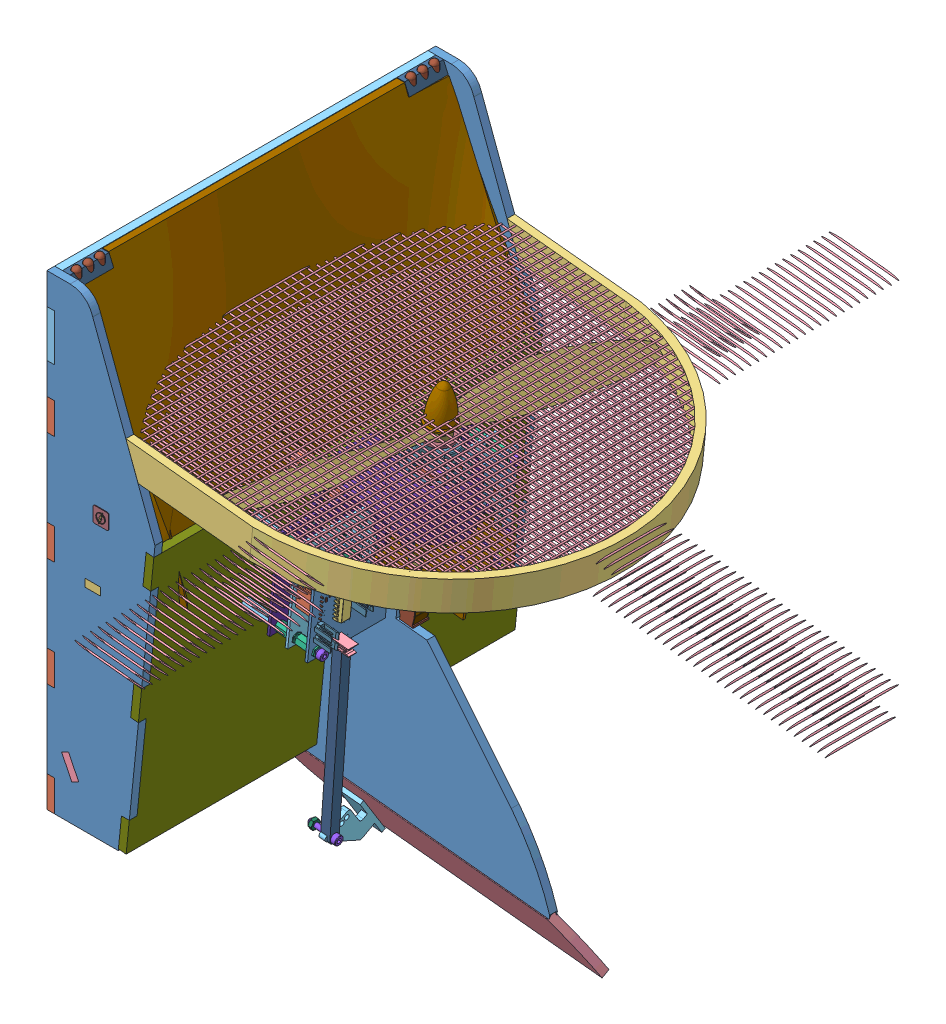
SolidWorks assembly AssTotaleSimu8, configuration Défaut. Lengths in mm. (continued)
Components (placement in the parent): (continued)
- AssStructSimu-1: AssStructSimu [Défaut] at (-125.7658 -1.8483 624.6548) x (1 0 0) z (0 0 -1) size (253.25 324.59 251.6) (continued)
  - AssCarte-1: AssCarte [Défaut] at (-42.8534 32.2132 302.028) x (-0.101852 0.9948 0) z (0.9948 0.101852 0) size (67.15 130.57 98.45) (continued)
    - carte_onduleur_v4-1: carte_onduleur_v4 [Défaut] at (-25.7639 0.8332 112.9379) size (66.52 130.57 82.34) (continued)
      - CON_IO1-1: CON_IO1 [Défaut] at (-11.3 12.1 0.803) x (0 -1 0) z (0 0 1) size (16.74 30.7 57.5) (continued)
        - Open CASCADE STEP translator 6.8 1.3.1-1: Open CASCADE STEP translator 6.8 1.3.1 [Défaut] at origin size (16.74 30.7 57.5) (continued)
          - Body_1_2-1: Body_1_2 [Défaut] at (-3 -15 8) x (0 -1 0) z (-1 0 0) size (30.7 57.5 16.74) (continued)
            - 57-1: 57 [Défaut] at (-15.3 2.7 -0.803) x (0 -1 0) z (0 0 -1) size (10.36 15.24 6.14) (continued)
              - =_[0_1_1_47]-1: =_[0_1_1_47] [Défaut] at origin size (10.36 15.24 6.14) (continued)
                - 55-1: 55 [Défaut] at (1.8 -1.2 3) x (1 0 0) z (0 1 0) size (10.36 6.14 15.24) (continued)
                  - 54-2: 54 [Défaut] at (0 0 -7.62) size (10.36 6.14 7.62) (continued)
                    - 52-2: 52 [Défaut] at (0 0 -2.54) size (10.36 6.14 2.54)
                      - 48-1: 48 [Défaut] at origin size (8.4 2.54 2.54)
                      - 49-1: 49 [Défaut] at (-0.0461 1.2682 1.27) x (0 0 -1) z (0.999998 -0.002105 0) size (1.95 5.07 7.58)
                    - 52-3: 52 [Défaut] at (0 0 -5.08) size (10.36 6.14 2.54)
                      - 48-1: 48 [Défaut] at origin size (8.4 2.54 2.54)
                      - 49-1: 49 [Défaut] at (-0.0461 1.2682 1.27) x (0 0 -1) z (0.999998 -0.002105 0) size (1.95 5.07 7.58)
            - 59-1: 59 [Défaut] at (-26.5 31 0.803) x (0 -1 0) z (0 0 1) size (2.34 1.04 0.5)
              - =_[0_1_1_42]-1: =_[0_1_1_42] [Défaut] at origin size (2.34 1.04 0.5)
                - 43-1: 43 [Défaut] at origin size (2.29 1.04 0.43)
                - 44-1: 44 [Défaut] at (0.3048 0 0) x (-1 0 0) z (0 0 1) size (0.51 1.02 0.5)
                - 45-1: 45 [Défaut] at origin size (0.51 1.02 0.5)
            - 61-1: 61 [Défaut] at (-21.6 17.8 0.803) x (-1 0 0) z (0 0 1) size (2.34 1.04 0.5)
              - =_[0_1_1_42]-1: =_[0_1_1_42] [Défaut] at origin size (2.34 1.04 0.5)
                - 43-1: 43 [Défaut] at origin size (2.29 1.04 0.43)
                - 44-1: 44 [Défaut] at (0.3048 0 0) x (-1 0 0) z (0 0 1) size (0.51 1.02 0.5)
                - 45-1: 45 [Défaut] at origin size (0.51 1.02 0.5)
            - 64-1: 64 [Défaut] at (-3.3 17.6 0.803) x (0 -1 0) z (0 0 1) size (8.01 8 14.24)
              - =_[0_1_1_56]-1: =_[0_1_1_56] [Défaut] at origin size (8.01 8 14.24)
                - 62-1: 62 [Défaut] at (1.8 0 0) x (1 0 0) z (0 -1 0) size (8.01 14.24 8)
      - CON_IO2-1: CON_IO2 [Défaut] at (-11.3 -2.7 0.803) x (0 -1 0) z (0 0 1) size (16.74 30.7 57.5)
        - Open CASCADE STEP translator 6.8 1.4.1-1: Open CASCADE STEP translator 6.8 1.4.1 [Défaut] at origin size (16.74 30.7 57.5)
          - Body_1_2-1: Body_1_2 [Défaut] at (-3 -15 8) x (0 -1 0) z (-1 0 0) size (30.7 57.5 16.74)
            - 1-1: 1 [Défaut] at origin size (30 50 1.61)
            - 10-1: 10 [Défaut] at (-14.395 31.0465 0.803) x (-1 0 0) z (0 0 1) size (5.59 6.35 1.11)
              - =_[0_1_1_4]-1: =_[0_1_1_4] [Défaut] at origin size (5.59 6.35 1.11)
                - 11-1: 11 [Défaut] at (2 3.3 0) x (-1 0 0) z (0 0 1) size (5.59 6.35 1.11)
                  - =_[0_1_1_3]_2-1: =_[0_1_1_3]_2 [Défaut] at origin size (0.44 0.55 0.36)
                  - =_[0_1_1_4]_2-1: =_[0_1_1_4]_2 [Défaut] at origin size (5.59 4.15 0.36)
                  - =_[0_1_1_5]_2-1: =_[0_1_1_5]_2 [Défaut] at origin size (5.35 6.1 1.1)
                  - =_[0_1_1_6]-1: =_[0_1_1_6] [Défaut] at origin size (0.44 0.55 0.36)
                  - =_[0_1_1_7]-1: =_[0_1_1_7] [Défaut] at origin size (0.44 0.55 0.36)
                  - =_[0_1_1_8]-1: =_[0_1_1_8] [Défaut] at origin size (0.44 0.55 0.36)
            - 13-1: 13 [Défaut] at (-12.62 16.6 -0.803) x (-1 0 0) z (0 0 -1) size (5.59 6.35 1.11)
              - =_[0_1_1_13]-1: =_[0_1_1_13] [Défaut] at origin size (5.59 6.35 1.11)
                - 11-1: 11 [Défaut] at (2 3.3 0) x (-1 0 0) z (0 0 1) size (5.59 6.35 1.11)
                  - =_[0_1_1_3]_2-1: =_[0_1_1_3]_2 [Défaut] at origin size (0.44 0.55 0.36)
                  - =_[0_1_1_4]_2-1: =_[0_1_1_4]_2 [Défaut] at origin size (5.59 4.15 0.36)
                  - =_[0_1_1_5]_2-1: =_[0_1_1_5]_2 [Défaut] at origin size (5.35 6.1 1.1)
                  - =_[0_1_1_6]-1: =_[0_1_1_6] [Défaut] at origin size (0.44 0.55 0.36)
                  - =_[0_1_1_7]-1: =_[0_1_1_7] [Défaut] at origin size (0.44 0.55 0.36)
                  - =_[0_1_1_8]-1: =_[0_1_1_8] [Défaut] at origin size (0.44 0.55 0.36)
            - 16-1: 16 [Défaut] at (-4.2 24.2 0.803) x (-1 0 0) z (0 0 1) size (12.8 0.5 13)
              - =_[0_1_1_15]-1: =_[0_1_1_15] [Défaut] at origin size (12.8 0.5 13)
                - 17-1: 17 [Défaut] at (2.7 0 0) x (1 0 0) z (0 -1 0) size (12.8 13 0.5)
            - 19-1: 19 [Défaut] at (-4.1 6.8 0.803) x (-1 0 0) z (0 0 1) size (12.8 0.5 13)
              - =_[0_1_1_18]-1: =_[0_1_1_18] [Défaut] at origin size (12.8 0.5 13)
                - 17-1: 17 [Défaut] at (2.7 0 0) x (1 0 0) z (0 -1 0) size (12.8 13 0.5)
            - 24-1: 24 [Défaut] at (-8.1 16.5 -0.803) x (0 1 0) z (0 0 -1) size (7.75 5.13 1.17)
              - =_[0_1_1_20]-1: =_[0_1_1_20] [Défaut] at origin size (7.75 5.13 1.17)
                - 20-1: 20 [Défaut] at origin size (7.59 5.13 1.07)
                - 21-1: 21 [Défaut] at (-14.478 0 0) x (-1 0 0) z (0 0 1) size (0.76 5.08 1.17)
                - 22-1: 22 [Défaut] at origin size (0.76 5.08 1.17)
            - 35-1: 35 [Défaut] at (-25.3 25.5 0.803) x (0 -1 0) z (0 0 1) size (6.05 5.2 1.7)
              - =_[0_1_1_25]-1: =_[0_1_1_25] [Défaut] at origin size (6.05 5.2 1.7)
                - 25-1: 25 [Défaut] at origin size (4.3 5.2 1.53)
                - 26-1: 26 [Défaut] at origin size (0.88 0.51 1.06)
                - 27-1: 27 [Défaut] at origin size (0.88 0.51 1.06)
                - 28-1: 28 [Défaut] at origin size (0.88 0.51 1.06)
                - 29-1: 29 [Défaut] at origin size (0.88 0.51 1.06)
                - 30-1: 30 [Défaut] at (11.6 -5.08 0) x (-1 0 0) z (0 0 1) size (0.87 0.51 1.06)
                - 31-1: 31 [Défaut] at (11.6 -2.54 0) x (-1 0 0) z (0 0 1) size (0.87 0.51 1.06)
                - 32-1: 32 [Défaut] at (11.6 0 0) x (-1 0 0) z (0 0 1) size (0.87 0.51 1.06)
                - 33-1: 33 [Défaut] at (11.6 2.54 0) x (-1 0 0) z (0 0 1) size (0.87 0.51 1.06)
            - 40-1: 40 [Défaut] at (-27.6 27.2 0.803) size (2.34 1.04 0.5)
              - =_[0_1_1_36]-1: =_[0_1_1_36] [Défaut] at origin size (2.34 1.04 0.5)
                - 36-1: 36 [Défaut] at origin size (2.29 1.04 0.43)
                - 37-1: 37 [Défaut] at (0.3048 0 0) x (-1 0 0) z (0 0 1) size (0.51 1.02 0.5)
                - 38-1: 38 [Défaut] at origin size (0.51 1.02 0.5)
            - 42-1: 42 [Défaut] at (-22.1 21.6 0.803) x (0 1 0) z (0 0 1) size (2.34 1.04 0.5)
              - =_[0_1_1_36]-1: =_[0_1_1_36] [Défaut] at origin size (2.34 1.04 0.5)
                - 36-1: 36 [Défaut] at origin size (2.29 1.04 0.43)
                - 37-1: 37 [Défaut] at (0.3048 0 0) x (-1 0 0) z (0 0 1) size (0.51 1.02 0.5)
                - 38-1: 38 [Défaut] at origin size (0.51 1.02 0.5)
            - 47-1: 47 [Défaut] at (-14.7664 14.5 -0.803) x (-1 0 0) z (0 0 -1) size (2.34 1.04 0.5)
              - =_[0_1_1_42]-1: =_[0_1_1_42] [Défaut] at origin size (2.34 1.04 0.5)
                - 43-1: 43 [Défaut] at origin size (2.29 1.04 0.43)
                - 44-1: 44 [Défaut] at (0.3048 0 0) x (-1 0 0) z (0 0 1) size (0.51 1.02 0.5)
                - 45-1: 45 [Défaut] at origin size (0.51 1.02 0.5)
            - 57-1: 57 [Défaut] at (-15.3 2.7 -0.803) x (0 -1 0) z (0 0 -1) size (10.36 15.24 6.14)
              - =_[0_1_1_47]-1: =_[0_1_1_47] [Défaut] at origin size (10.36 15.24 6.14)
                - 55-1: 55 [Défaut] at (1.8 -1.2 3) x (1 0 0) z (0 1 0) size (10.36 6.14 15.24)
                  - 54-1: 54 [Défaut] at origin size (10.36 6.14 7.62)
                    - 52-1: 52 [Défaut] at origin size (10.36 6.14 2.54)
                      - 48-1: 48 [Défaut] at origin size (8.4 2.54 2.54)
                      - 49-1: 49 [Défaut] at (-0.0461 1.2682 1.27) x (0 0 -1) z (0.999998 -0.002105 0) size (1.95 5.07 7.58)
                    - 52-2: 52 [Défaut] at (0 0 -2.54) size (10.36 6.14 2.54)
                      - 48-1: 48 [Défaut] at origin size (8.4 2.54 2.54)
                      - 49-1: 49 [Défaut] at (-0.0461 1.2682 1.27) x (0 0 -1) z (0.999998 -0.002105 0) size (1.95 5.07 7.58)
                    - 52-3: 52 [Défaut] at (0 0 -5.08) size (10.36 6.14 2.54)
                      - 48-1: 48 [Défaut] at origin size (8.4 2.54 2.54)
                      - 49-1: 49 [Défaut] at (-0.0461 1.2682 1.27) x (0 0 -1) z (0.999998 -0.002105 0) size (1.95 5.07 7.58)
                  - 54-2: 54 [Défaut] at (0 0 -7.62) size (10.36 6.14 7.62)
                    - 52-1: 52 [Défaut] at origin size (10.36 6.14 2.54)
                      - 48-1: 48 [Défaut] at origin size (8.4 2.54 2.54)
                      - 49-1: 49 [Défaut] at (-0.0461 1.2682 1.27) x (0 0 -1) z (0.999998 -0.002105 0) size (1.95 5.07 7.58)
                    - 52-2: 52 [Défaut] at (0 0 -2.54) size (10.36 6.14 2.54)
                      - 48-1: 48 [Défaut] at origin size (8.4 2.54 2.54)
                      - 49-1: 49 [Défaut] at (-0.0461 1.2682 1.27) x (0 0 -1) z (0.999998 -0.002105 0) size (1.95 5.07 7.58)
                    - 52-3: 52 [Défaut] at (0 0 -5.08) size (10.36 6.14 2.54)
                      - 48-1: 48 [Défaut] at origin size (8.4 2.54 2.54)
                      - 49-1: 49 [Défaut] at (-0.0461 1.2682 1.27) x (0 0 -1) z (0.999998 -0.002105 0) size (1.95 5.07 7.58)
            - 59-1: 59 [Défaut] at (-26.5 31 0.803) x (0 -1 0) z (0 0 1) size (2.34 1.04 0.5)
              - =_[0_1_1_42]-1: =_[0_1_1_42] [Défaut] at origin size (2.34 1.04 0.5)
                - 43-1: 43 [Défaut] at origin size (2.29 1.04 0.43)
                - 44-1: 44 [Défaut] at (0.3048 0 0) x (-1 0 0) z (0 0 1) size (0.51 1.02 0.5)
                - 45-1: 45 [Défaut] at origin size (0.51 1.02 0.5)
            - 61-1: 61 [Défaut] at (-21.6 17.8 0.803) x (-1 0 0) z (0 0 1) size (2.34 1.04 0.5)
              - =_[0_1_1_42]-1: =_[0_1_1_42] [Défaut] at origin size (2.34 1.04 0.5)
                - 43-1: 43 [Défaut] at origin size (2.29 1.04 0.43)
                - 44-1: 44 [Défaut] at (0.3048 0 0) x (-1 0 0) z (0 0 1) size (0.51 1.02 0.5)
                - 45-1: 45 [Défaut] at origin size (0.51 1.02 0.5)
            - 64-1: 64 [Défaut] at (-3.3 17.6 0.803) x (0 -1 0) z (0 0 1) size (8.01 8 14.24)
              - =_[0_1_1_56]-1: =_[0_1_1_56] [Défaut] at origin size (8.01 8 14.24)
                - 62-1: 62 [Défaut] at (1.8 0 0) x (1 0 0) z (0 -1 0) size (8.01 14.24 8)
      - CON_IO3-1: CON_IO3 [Défaut] at (-11.3 -17.7 0.803) x (0 -1 0) z (0 0 1) size (16.74 30.7 57.5)
        - Open CASCADE STEP translator 6.8 1.5.1-1: Open CASCADE STEP translator 6.8 1.5.1 [Défaut] at origin size (16.74 30.7 57.5)
          - Body_1_2-1: Body_1_2 [Défaut] at (-3 -15 8) x (0 -1 0) z (-1 0 0) size (30.7 57.5 16.74)
            - 1-1: 1 [Défaut] at origin size (30 50 1.61)
            - 10-1: 10 [Défaut] at (-14.395 31.0465 0.803) x (-1 0 0) z (0 0 1) size (5.59 6.35 1.11)
              - =_[0_1_1_4]-1: =_[0_1_1_4] [Défaut] at origin size (5.59 6.35 1.11)
                - 11-1: 11 [Défaut] at (2 3.3 0) x (-1 0 0) z (0 0 1) size (5.59 6.35 1.11)
                  - =_[0_1_1_3]_2-1: =_[0_1_1_3]_2 [Défaut] at origin size (0.44 0.55 0.36)
                  - =_[0_1_1_4]_2-1: =_[0_1_1_4]_2 [Défaut] at origin size (5.59 4.15 0.36)
                  - =_[0_1_1_5]_2-1: =_[0_1_1_5]_2 [Défaut] at origin size (5.35 6.1 1.1)
                  - =_[0_1_1_6]-1: =_[0_1_1_6] [Défaut] at origin size (0.44 0.55 0.36)
                  - =_[0_1_1_7]-1: =_[0_1_1_7] [Défaut] at origin size (0.44 0.55 0.36)
                  - =_[0_1_1_8]-1: =_[0_1_1_8] [Défaut] at origin size (0.44 0.55 0.36)
            - 13-1: 13 [Défaut] at (-12.62 16.6 -0.803) x (-1 0 0) z (0 0 -1) size (5.59 6.35 1.11)
              - =_[0_1_1_13]-1: =_[0_1_1_13] [Défaut] at origin size (5.59 6.35 1.11)
                - 11-1: 11 [Défaut] at (2 3.3 0) x (-1 0 0) z (0 0 1) size (5.59 6.35 1.11)
                  - =_[0_1_1_3]_2-1: =_[0_1_1_3]_2 [Défaut] at origin size (0.44 0.55 0.36)
                  - =_[0_1_1_4]_2-1: =_[0_1_1_4]_2 [Défaut] at origin size (5.59 4.15 0.36)
                  - =_[0_1_1_5]_2-1: =_[0_1_1_5]_2 [Défaut] at origin size (5.35 6.1 1.1)
                  - =_[0_1_1_6]-1: =_[0_1_1_6] [Défaut] at origin size (0.44 0.55 0.36)
                  - =_[0_1_1_7]-1: =_[0_1_1_7] [Défaut] at origin size (0.44 0.55 0.36)
                  - =_[0_1_1_8]-1: =_[0_1_1_8] [Défaut] at origin size (0.44 0.55 0.36)
            - 16-1: 16 [Défaut] at (-4.2 24.2 0.803) x (-1 0 0) z (0 0 1) size (12.8 0.5 13)
              - =_[0_1_1_15]-1: =_[0_1_1_15] [Défaut] at origin size (12.8 0.5 13)
                - 17-1: 17 [Défaut] at (2.7 0 0) x (1 0 0) z (0 -1 0) size (12.8 13 0.5)
            - 19-1: 19 [Défaut] at (-4.1 6.8 0.803) x (-1 0 0) z (0 0 1) size (12.8 0.5 13)
              - =_[0_1_1_18]-1: =_[0_1_1_18] [Défaut] at origin size (12.8 0.5 13)
                - 17-1: 17 [Défaut] at (2.7 0 0) x (1 0 0) z (0 -1 0) size (12.8 13 0.5)
            - 24-1: 24 [Défaut] at (-8.1 16.5 -0.803) x (0 1 0) z (0 0 -1) size (7.75 5.13 1.17)
              - =_[0_1_1_20]-1: =_[0_1_1_20] [Défaut] at origin size (7.75 5.13 1.17)
                - 20-1: 20 [Défaut] at origin size (7.59 5.13 1.07)
                - 21-1: 21 [Défaut] at (-14.478 0 0) x (-1 0 0) z (0 0 1) size (0.76 5.08 1.17)
                - 22-1: 22 [Défaut] at origin size (0.76 5.08 1.17)
            - 35-1: 35 [Défaut] at (-25.3 25.5 0.803) x (0 -1 0) z (0 0 1) size (6.05 5.2 1.7)
              - =_[0_1_1_25]-1: =_[0_1_1_25] [Défaut] at origin size (6.05 5.2 1.7)
                - 25-1: 25 [Défaut] at origin size (4.3 5.2 1.53)
                - 26-1: 26 [Défaut] at origin size (0.88 0.51 1.06)
                - 27-1: 27 [Défaut] at origin size (0.88 0.51 1.06)
                - 28-1: 28 [Défaut] at origin size (0.88 0.51 1.06)
                - 29-1: 29 [Défaut] at origin size (0.88 0.51 1.06)
                - 30-1: 30 [Défaut] at (11.6 -5.08 0) x (-1 0 0) z (0 0 1) size (0.87 0.51 1.06)
                - 31-1: 31 [Défaut] at (11.6 -2.54 0) x (-1 0 0) z (0 0 1) size (0.87 0.51 1.06)
                - 32-1: 32 [Défaut] at (11.6 0 0) x (-1 0 0) z (0 0 1) size (0.87 0.51 1.06)
                - 33-1: 33 [Défaut] at (11.6 2.54 0) x (-1 0 0) z (0 0 1) size (0.87 0.51 1.06)
            - 40-1: 40 [Défaut] at (-27.6 27.2 0.803) size (2.34 1.04 0.5)
              - =_[0_1_1_36]-1: =_[0_1_1_36] [Défaut] at origin size (2.34 1.04 0.5)
                - 36-1: 36 [Défaut] at origin size (2.29 1.04 0.43)
                - 37-1: 37 [Défaut] at (0.3048 0 0) x (-1 0 0) z (0 0 1) size (0.51 1.02 0.5)
                - 38-1: 38 [Défaut] at origin size (0.51 1.02 0.5)
            - 42-1: 42 [Défaut] at (-22.1 21.6 0.803) x (0 1 0) z (0 0 1) size (2.34 1.04 0.5)
              - =_[0_1_1_36]-1: =_[0_1_1_36] [Défaut] at origin size (2.34 1.04 0.5)
                - 36-1: 36 [Défaut] at origin size (2.29 1.04 0.43)
                - 37-1: 37 [Défaut] at (0.3048 0 0) x (-1 0 0) z (0 0 1) size (0.51 1.02 0.5)
                - 38-1: 38 [Défaut] at origin size (0.51 1.02 0.5)
            - 47-1: 47 [Défaut] at (-14.7664 14.5 -0.803) x (-1 0 0) z (0 0 -1) size (2.34 1.04 0.5)
              - =_[0_1_1_42]-1: =_[0_1_1_42] [Défaut] at origin size (2.34 1.04 0.5)
                - 43-1: 43 [Défaut] at origin size (2.29 1.04 0.43)
                - 44-1: 44 [Défaut] at (0.3048 0 0) x (-1 0 0) z (0 0 1) size (0.51 1.02 0.5)
                - 45-1: 45 [Défaut] at origin size (0.51 1.02 0.5)
            - 57-1: 57 [Défaut] at (-15.3 2.7 -0.803) x (0 -1 0) z (0 0 -1) size (10.36 15.24 6.14)
              - =_[0_1_1_47]-1: =_[0_1_1_47] [Défaut] at origin size (10.36 15.24 6.14)
                - 55-1: 55 [Défaut] at (1.8 -1.2 3) x (1 0 0) z (0 1 0) size (10.36 6.14 15.24)
                  - 54-1: 54 [Défaut] at origin size (10.36 6.14 7.62)
                    - 52-1: 52 [Défaut] at origin size (10.36 6.14 2.54)
                      - 48-1: 48 [Défaut] at origin size (8.4 2.54 2.54)
                      - 49-1: 49 [Défaut] at (-0.0461 1.2682 1.27) x (0 0 -1) z (0.999998 -0.002105 0) size (1.95 5.07 7.58)
                    - 52-2: 52 [Défaut] at (0 0 -2.54) size (10.36 6.14 2.54)
                      - 48-1: 48 [Défaut] at origin size (8.4 2.54 2.54)
                      - 49-1: 49 [Défaut] at (-0.0461 1.2682 1.27) x (0 0 -1) z (0.999998 -0.002105 0) size (1.95 5.07 7.58)
                    - 52-3: 52 [Défaut] at (0 0 -5.08) size (10.36 6.14 2.54)
                      - 48-1: 48 [Défaut] at origin size (8.4 2.54 2.54)
                      - 49-1: 49 [Défaut] at (-0.0461 1.2682 1.27) x (0 0 -1) z (0.999998 -0.002105 0) size (1.95 5.07 7.58)
                  - 54-2: 54 [Défaut] at (0 0 -7.62) size (10.36 6.14 7.62)
                    - 52-1: 52 [Défaut] at origin size (10.36 6.14 2.54)
                      - 48-1: 48 [Défaut] at origin size (8.4 2.54 2.54)
                      - 49-1: 49 [Défaut] at (-0.0461 1.2682 1.27) x (0 0 -1) z (0.999998 -0.002105 0) size (1.95 5.07 7.58)
                    - 52-2: 52 [Défaut] at (0 0 -2.54) size (10.36 6.14 2.54)
                      - 48-1: 48 [Défaut] at origin size (8.4 2.54 2.54)
                      - 49-1: 49 [Défaut] at (-0.0461 1.2682 1.27) x (0 0 -1) z (0.999998 -0.002105 0) size (1.95 5.07 7.58)
                    - 52-3: 52 [Défaut] at (0 0 -5.08) size (10.36 6.14 2.54)
                      - 48-1: 48 [Défaut] at origin size (8.4 2.54 2.54)
                      - 49-1: 49 [Défaut] at (-0.0461 1.2682 1.27) x (0 0 -1) z (0.999998 -0.002105 0) size (1.95 5.07 7.58)
            - 59-1: 59 [Défaut] at (-26.5 31 0.803) x (0 -1 0) z (0 0 1) size (2.34 1.04 0.5)
              - =_[0_1_1_42]-1: =_[0_1_1_42] [Défaut] at origin size (2.34 1.04 0.5)
                - 43-1: 43 [Défaut] at origin size (2.29 1.04 0.43)
                - 44-1: 44 [Défaut] at (0.3048 0 0) x (-1 0 0) z (0 0 1) size (0.51 1.02 0.5)
                - 45-1: 45 [Défaut] at origin size (0.51 1.02 0.5)
            - 61-1: 61 [Défaut] at (-21.6 17.8 0.803) x (-1 0 0) z (0 0 1) size (2.34 1.04 0.5)
              - =_[0_1_1_42]-1: =_[0_1_1_42] [Défaut] at origin size (2.34 1.04 0.5)
                - 43-1: 43 [Défaut] at origin size (2.29 1.04 0.43)
                - 44-1: 44 [Défaut] at (0.3048 0 0) x (-1 0 0) z (0 0 1) size (0.51 1.02 0.5)
                - 45-1: 45 [Défaut] at origin size (0.51 1.02 0.5)
            - 64-1: 64 [Défaut] at (-3.3 17.6 0.803) x (0 -1 0) z (0 0 1) size (8.01 8 14.24)
              - =_[0_1_1_56]-1: =_[0_1_1_56] [Défaut] at origin size (8.01 8 14.24)
                - 62-1: 62 [Défaut] at (1.8 0 0) x (1 0 0) z (0 -1 0) size (8.01 14.24 8)
      - C1_1-1: C1_1 [Défaut] at (-20.6336 6.4 -0.803) x (1 0 0) z (0 0 -1) size (2.34 1.04 0.5)
        - Open CASCADE STEP translator 6.8 1.6.1-1: Open CASCADE STEP translator 6.8 1.6.1 [Défaut] at origin size (2.34 1.04 0.5)
          - Body_1-1: Body_1 [Défaut] at origin size (2.29 1.04 0.43)
          - Pin_1-1: Pin_1 [Défaut] at (0.3048 0 0) x (-1 0 0) z (0 0 1) size (0.51 1.02 0.5)
          - Pin_2-1: Pin_2 [Défaut] at origin size (0.51 1.02 0.5)
      - C1_2-1: C1_2 [Défaut] at (-24.2 6.4 -0.803) x (1 0 0) z (0 0 -1) size (2.34 1.04 0.5)
        - Open CASCADE STEP translator 6.8 1.6.1-1: Open CASCADE STEP translator 6.8 1.6.1 [Défaut] at origin size (2.34 1.04 0.5)
          - Body_1-1: Body_1 [Défaut] at origin size (2.29 1.04 0.43)
          - Pin_1-1: Pin_1 [Défaut] at (0.3048 0 0) x (-1 0 0) z (0 0 1) size (0.51 1.02 0.5)
          - Pin_2-1: Pin_2 [Défaut] at origin size (0.51 1.02 0.5)
      - C_F-1: C_F [Défaut] at (-16.2432 4.45 -0.803) x (0 -1 0) z (0 0 -1) size (2.34 1.04 0.5)
        - Open CASCADE STEP translator 6.8 1.6.1-1: Open CASCADE STEP translator 6.8 1.6.1 [Défaut] at origin size (2.34 1.04 0.5)
          - Body_1-1: Body_1 [Défaut] at origin size (2.29 1.04 0.43)
          - Pin_1-1: Pin_1 [Défaut] at (0.3048 0 0) x (-1 0 0) z (0 0 1) size (0.51 1.02 0.5)
          - Pin_2-1: Pin_2 [Défaut] at origin size (0.51 1.02 0.5)
      - D_LED_STATE1-1: D_LED_STATE1 [Défaut] at (-6.8906 -21.6 0.803) size (2.34 1.04 0.5)
        - Open CASCADE STEP translator 6.8 1.6.1-1: Open CASCADE STEP translator 6.8 1.6.1 [Défaut] at origin size (2.34 1.04 0.5)
          - Body_1-1: Body_1 [Défaut] at origin size (2.29 1.04 0.43)
          - Pin_1-1: Pin_1 [Défaut] at (0.3048 0 0) x (-1 0 0) z (0 0 1) size (0.51 1.02 0.5)
          - Pin_2-1: Pin_2 [Défaut] at origin size (0.51 1.02 0.5)
      - PICKIT-1: PICKIT [Défaut] at (-24.1 -30.5 0.803) size (15.24 5 14.3)
        - Open CASCADE STEP translator 6.8 1.10.1-1: Open CASCADE STEP translator 6.8 1.10.1 [Défaut] at origin size (15.24 5 14.3)
          - Body_1_2-1: Body_1_2 [Défaut] at (6.3 0 12) size (15.24 5 14.3)
      - C_DEC_CUR-1: C_DEC_CUR [Défaut] at (-8.9496 5.7572 -0.803) x (0 1 0) z (0 0 -1) size (2.34 1.04 0.5)
        - Open CASCADE STEP translator 6.8 1.6.1-1: Open CASCADE STEP translator 6.8 1.6.1 [Défaut] at origin size (2.34 1.04 0.5)
          - Body_1-1: Body_1 [Défaut] at origin size (2.29 1.04 0.43)
          - Pin_1-1: Pin_1 [Défaut] at (0.3048 0 0) x (-1 0 0) z (0 0 1) size (0.51 1.02 0.5)
          - Pin_2-1: Pin_2 [Défaut] at origin size (0.51 1.02 0.5)
      - R_F-1: R_F [Défaut] at (-14.65 4.4432 -0.803) x (0 -1 0) z (0 0 -1) size (2.34 1.04 0.5)
        - Open CASCADE STEP translator 6.8 1.12.1-1: Open CASCADE STEP translator 6.8 1.12.1 [Défaut] at origin size (2.34 1.04 0.5)
          - Body_1_3-1: Body_1_3 [Défaut] at origin size (2.29 1.04 0.43)
          - Pin_1_2-1: Pin_1_2 [Défaut] at (0.3048 0 0) x (-1 0 0) z (0 0 1) size (0.51 1.02 0.5)
          - Pin_2_2-1: Pin_2_2 [Défaut] at origin size (0.51 1.02 0.5)
      - R_GAIN1-1: R_GAIN1 [Défaut] at (-13.95 5.7568 -0.803) x (0 1 0) z (0 0 -1) size (2.34 1.04 0.5)
        - Open CASCADE STEP translator 6.8 1.12.1-1: Open CASCADE STEP translator 6.8 1.12.1 [Défaut] at origin size (2.34 1.04 0.5)
          - Body_1_3-1: Body_1_3 [Défaut] at origin size (2.29 1.04 0.43)
          - Pin_1_2-1: Pin_1_2 [Défaut] at (0.3048 0 0) x (-1 0 0) z (0 0 1) size (0.51 1.02 0.5)
          - Pin_2_2-1: Pin_2_2 [Défaut] at origin size (0.51 1.02 0.5)
      - R_GAIN2-1: R_GAIN2 [Défaut] at (-15.65 7.9176 -0.803) x (0 -1 0) z (0 0 -1) size (2.34 1.04 0.5)
        - Open CASCADE STEP translator 6.8 1.12.1-1: Open CASCADE STEP translator 6.8 1.12.1 [Défaut] at origin size (2.34 1.04 0.5)
          - Body_1_3-1: Body_1_3 [Défaut] at origin size (2.29 1.04 0.43)
          - Pin_1_2-1: Pin_1_2 [Défaut] at (0.3048 0 0) x (-1 0 0) z (0 0 1) size (0.51 1.02 0.5)
          - Pin_2_2-1: Pin_2_2 [Défaut] at origin size (0.51 1.02 0.5)
      - R_LED_STATE1-1: R_LED_STATE1 [Défaut] at (-6.9242 -19.9 0.803) size (2.34 1.04 0.5)
        - Open CASCADE STEP translator 6.8 1.12.1-1: Open CASCADE STEP translator 6.8 1.12.1 [Défaut] at origin size (2.34 1.04 0.5)
          - Body_1_3-1: Body_1_3 [Défaut] at origin size (2.29 1.04 0.43)
          - Pin_1_2-1: Pin_1_2 [Défaut] at (0.3048 0 0) x (-1 0 0) z (0 0 1) size (0.51 1.02 0.5)
          - Pin_2_2-1: Pin_2_2 [Défaut] at origin size (0.51 1.02 0.5)
      - R_RESET1-1: R_RESET1 [Défaut] at (-23 7.9 0.803) size (2.34 1.04 0.5)
        - Open CASCADE STEP translator 6.8 1.12.1-1: Open CASCADE STEP translator 6.8 1.12.1 [Défaut] at origin size (2.34 1.04 0.5)
          - Body_1_3-1: Body_1_3 [Défaut] at origin size (2.29 1.04 0.43)
          - Pin_1_2-1: Pin_1_2 [Défaut] at (0.3048 0 0) x (-1 0 0) z (0 0 1) size (0.51 1.02 0.5)
          - Pin_2_2-1: Pin_2_2 [Défaut] at origin size (0.51 1.02 0.5)
      - U_DSPIC-1: U_DSPIC [Défaut] at (1.863 -2.61 0.803) size (7.92 35.56 7.75)
        - Open CASCADE STEP translator 6.8 1.17.1-1: Open CASCADE STEP translator 6.8 1.17.1 [Défaut] at origin size (7.92 35.56 7.75)
          - Body_1_4-1: Body_1_4 [Défaut] at (0 -0.2 4) x (1 0 0) z (0 -1 0) size (7.92 7.75 35.56)
      - C_DEC_DSPIC-1: C_DEC_DSPIC [Défaut] at (7.7 -8.8 -0.803) x (0 1 0) z (0 0 -1) size (2.34 1.04 0.5)
        - Open CASCADE STEP translator 6.8 1.6.1-1: Open CASCADE STEP translator 6.8 1.6.1 [Défaut] at origin size (2.34 1.04 0.5)
          - Body_1-1: Body_1 [Défaut] at origin size (2.29 1.04 0.43)
          - Pin_1-1: Pin_1 [Défaut] at (0.3048 0 0) x (-1 0 0) z (0 0 1) size (0.51 1.02 0.5)
          - Pin_2-1: Pin_2 [Défaut] at origin size (0.51 1.02 0.5)
      - IN-1: IN [Défaut] at (24.3 -5.3 0.803) x (0 1 0) z (0 0 1) size (10.21 15.56 26.9)
        - Open CASCADE STEP translator 6.8 1.19.1-1: Open CASCADE STEP translator 6.8 1.19.1 [Défaut] at origin size (10.21 15.56 26.9)
          - Body_1_3-1: Body_1_3 [Défaut] at (-13.5 1.8 3) x (0 1 0) z (1 0 0) size (15.56 26.9 10.21)
            - Imported-1: Imported [Défaut] at (2.0451 -4.5908 20.9802) size (8.6 15.9 10.16)
            - Imported-2: Imported [Défaut] at (-1.6683 9.1092 15.9802) x (0 0 1) z (-1 0 0) size (10.1 18.2 15.1)
              - Imported_2-1: Imported_2 [Défaut] at origin size (10.1 18.2 15.1)
              - Imported_3-1: Imported_3 [Défaut] at origin size (3.43 12.4 4.99)
              - Imported_4-1: Imported_4 [Défaut] at origin size (3.43 12.4 4.99)
              - Imported_5-1: Imported_5 [Défaut] at origin size (3.9 4.9 7)
              - Imported_6-1: Imported_6 [Défaut] at origin size (3.9 4.9 7)
              - Imported_7-1: Imported_7 [Défaut] at origin size (3.8 3.8 6.92)
              - Imported_8-1: Imported_8 [Défaut] at origin size (3.8 3.8 6.92)
              - Imported_9-1: Imported_9 [Défaut] at origin size (9 2.4 14.2)
      - CARTE_CMD-1: CARTE_CMD [Défaut] at (25 57.2 0.803) size (60.1 130 26.71)
        - Open CASCADE STEP translator 6.8 1.20.1-1: Open CASCADE STEP translator 6.8 1.20.1 [Défaut] at origin size (60.1 130 26.71)
          - Body_1_4-1: Body_1_4 [Défaut] at (-55 5 12) size (60.1 130 26.71)
            - 1_2-1: 1_2 [Défaut] at origin size (60.1 130 1.61)
            - 4-1: 4 [Défaut] at (23.6 -124.9 0.803) x (0 1 0) z (0 0 1) size (5 15.24 14.3)
              - =_[0_1_1_4]_2-1: =_[0_1_1_4]_2 [Défaut] at origin size (5 15.24 14.3)
                - 5-1: 5 [Défaut] at (0 -6.5 -13) x (0 1 0) z (0 0 -1) size (15.24 5 14.3)
            - 7-1: 7 [Défaut] at (23.6 -5 0.803) x (0 1 0) z (0 0 1) size (5 15.24 14.3)
              - =_[0_1_1_7]-1: =_[0_1_1_7] [Défaut] at origin size (5 15.24 14.3)
                - 5-1: 5 [Défaut] at (0 -6.5 -13) x (0 1 0) z (0 0 -1) size (15.24 5 14.3)
            - 10_2-1: 10_2 [Défaut] at (18.4 -115.6 0.803) size (25.4 7.92 7.75)
              - =_[0_1_1_9]-1: =_[0_1_1_9] [Défaut] at origin size (25.4 7.92 7.75)
                - 8-1: 8 [Défaut] at (11.2 4 0) x (0 1 0) z (1 0 0) size (7.92 7.75 25.4)
            - 13_2-1: 13_2 [Défaut] at (55.4 -114.7 0.803) x (-1 0 0) z (0 0 1) size (5 7.62 14.3)
              - =_[0_1_1_12]-1: =_[0_1_1_12] [Défaut] at origin size (5 7.62 14.3)
                - 11-1: 11 [Défaut] at (0 -2.5 11) x (0 -1 0) z (0 0 1) size (7.62 5 14.3)
            - 25-1: 25 [Défaut] at (56.9 -12.8 0.803) x (-1 0 0) z (0 0 1) size (16.02 47.26 11.05)
              - =_[0_1_1_15]_2-1: =_[0_1_1_15]_2 [Défaut] at origin size (16.02 47.26 11.05)
                - 23-1: 23 [Défaut] at (-36.5 21 4) x (0 -1 0) z (1 0 0) size (47.26 11.05 16.02)
                  - 14-1: 14 [Défaut] at (-7.4961 -1.5352 42.5833) size (42.58 6.55 16.01)
                  - 22-1: 22 [Défaut] at (19.3039 2.3748 37.905) x (-1 0 0) z (0 0 -1) size (10.36 6.14 15.24)
                    - 21-1: 21 [Défaut] at origin size (10.36 6.14 7.62)
                      - 19_2-1: 19_2 [Défaut] at origin size (10.36 6.14 2.54)
                        - 15-1: 15 [Défaut] at origin size (8.4 2.54 2.54)
                        - 16-1: 16 [Défaut] at (-0.0461 1.2682 1.27) x (0 0 -1) z (0.999998 -0.002105 0) size (1.95 5.07 7.58)
                      - 19_2-2: 19_2 [Défaut] at (0 0 -2.54) size (10.36 6.14 2.54)
                        - 15-1: 15 [Défaut] at origin size (8.4 2.54 2.54)
                        - 16-1: 16 [Défaut] at (-0.0461 1.2682 1.27) x (0 0 -1) z (0.999998 -0.002105 0) size (1.95 5.07 7.58)
                      - 19_2-3: 19_2 [Défaut] at (0 0 -5.08) size (10.36 6.14 2.54)
                        - 15-1: 15 [Défaut] at origin size (8.4 2.54 2.54)
                        - 16-1: 16 [Défaut] at (-0.0461 1.2682 1.27) x (0 0 -1) z (0.999998 -0.002105 0) size (1.95 5.07 7.58)
                    - 21-2: 21 [Défaut] at (0 0 -7.62) size (10.36 6.14 7.62)
                      - 19_2-1: 19_2 [Défaut] at origin size (10.36 6.14 2.54)
                        - 15-1: 15 [Défaut] at origin size (8.4 2.54 2.54)
                        - 16-1: 16 [Défaut] at (-0.0461 1.2682 1.27) x (0 0 -1) z (0.999998 -0.002105 0) size (1.95 5.07 7.58)
                      - 19_2-2: 19_2 [Défaut] at (0 0 -2.54) size (10.36 6.14 2.54)
                        - 15-1: 15 [Défaut] at origin size (8.4 2.54 2.54)
                        - 16-1: 16 [Défaut] at (-0.0461 1.2682 1.27) x (0 0 -1) z (0.999998 -0.002105 0) size (1.95 5.07 7.58)
                      - 19_2-3: 19_2 [Défaut] at (0 0 -5.08) size (10.36 6.14 2.54)
                        - 15-1: 15 [Défaut] at origin size (8.4 2.54 2.54)
                        - 16-1: 16 [Défaut] at (-0.0461 1.2682 1.27) x (0 0 -1) z (0.999998 -0.002105 0) size (1.95 5.07 7.58)
            - 31-1: 31 [Défaut] at (12.9 -104.5 0.803) size (6.76 3.64 4.37)
              - =_[0_1_1_24]-1: =_[0_1_1_24] [Défaut] at origin size (6.76 3.64 4.37)
                - 29-1: 29 [Défaut] at (-0.3 -2 0) size (6.76 3.64 4.37)
                  - =_[0_1_1_3]_3-1: =_[0_1_1_3]_3 [Défaut] at origin size (6 3.64 4.37)
                  - =_[0_1_1_4]_3-1: =_[0_1_1_4]_3 [Défaut] at origin size (0.38 1 0.67)
                  - =_[0_1_1_5]_3-1: =_[0_1_1_5]_3 [Défaut] at origin size (0.38 1 0.67)
            - 36-1: 36 [Défaut] at (28.6 -12.2 0.803) x (0 -1 0) z (0 0 1) size (2.34 1.04 0.5)
              - =_[0_1_1_30]-1: =_[0_1_1_30] [Défaut] at origin size (2.34 1.04 0.5)
                - 32_2-1: 32_2 [Défaut] at origin size (2.29 1.04 0.43)
                - 33_2-1: 33_2 [Défaut] at (0.3048 0 0) x (-1 0 0) z (0 0 1) size (0.51 1.02 0.5)
                - 34-1: 34 [Défaut] at origin size (0.51 1.02 0.5)
            - 38-1: 38 [Défaut] at (23.7 -12.2 0.803) x (0 -1 0) z (0 0 1) size (2.34 1.04 0.5)
              - =_[0_1_1_30]-1: =_[0_1_1_30] [Défaut] at origin size (2.34 1.04 0.5)
                - 32_2-1: 32_2 [Défaut] at origin size (2.29 1.04 0.43)
                - 33_2-1: 33_2 [Défaut] at (0.3048 0 0) x (-1 0 0) z (0 0 1) size (0.51 1.02 0.5)
                - 34-1: 34 [Défaut] at origin size (0.51 1.02 0.5)
            - 40_2-1: 40_2 [Défaut] at (26.2 -12.2 0.803) x (0 -1 0) z (0 0 1) size (2.34 1.04 0.5)
              - =_[0_1_1_30]-1: =_[0_1_1_30] [Défaut] at origin size (2.34 1.04 0.5)
                - 32_2-1: 32_2 [Défaut] at origin size (2.29 1.04 0.43)
                - 33_2-1: 33_2 [Défaut] at (0.3048 0 0) x (-1 0 0) z (0 0 1) size (0.51 1.02 0.5)
                - 34-1: 34 [Défaut] at origin size (0.51 1.02 0.5)
            - 42_2-1: 42_2 [Défaut] at (24.4 -119.2 0.803) size (2.34 1.04 0.5)
              - =_[0_1_1_30]-1: =_[0_1_1_30] [Défaut] at origin size (2.34 1.04 0.5)
                - 32_2-1: 32_2 [Défaut] at origin size (2.29 1.04 0.43)
                - 33_2-1: 33_2 [Défaut] at (0.3048 0 0) x (-1 0 0) z (0 0 1) size (0.51 1.02 0.5)
                - 34-1: 34 [Défaut] at origin size (0.51 1.02 0.5)
            - 45-1: 45 [Défaut] at (46.4 -125 0.803) size (5.08 5 14.3)
              - =_[0_1_1_38]-1: =_[0_1_1_38] [Défaut] at origin size (5.08 5 14.3)
                - 190-1: 190 [Défaut] at (1.2 0 11) size (5.08 5 14.3)
            - 48-1: 48 [Défaut] at (40.1 -125 0.803) size (5.08 5 14.3)
              - =_[0_1_1_41]-1: =_[0_1_1_41] [Défaut] at origin size (5.08 5 14.3)
                - 190-1: 190 [Défaut] at (1.2 0 11) size (5.08 5 14.3)
            - 51-1: 51 [Défaut] at (6.4 -119.9 0.803) x (0 1 0) z (0 0 1) size (15.24 2.54 7.37)
              - =_[0_1_1_43]-1: =_[0_1_1_43] [Défaut] at origin size (15.24 2.54 7.37)
                - 49_2-1: 49_2 [Défaut] at (6.5 0 0) x (1 0 0) z (0 -1 0) size (15.24 7.37 2.54)
            - 57_2-1: 57_2 [Défaut] at (50.8796 -121.1 -0.803) x (-1 0 0) z (0 0 -1) size (2.54 1.98 0.64)
              - =_[0_1_1_46]-1: =_[0_1_1_46] [Défaut] at origin size (2.54 1.98 0.64)
                - 52-1: 52 [Défaut] at origin size (2.54 1.14 0.58)
                - 53-1: 53 [Défaut] x (0 -1 0) z (0 0 1) size (0.43 0.51 0.38)
                - 54-1: 54 [Défaut] at (1.8796 1.8796 0) x (0 -1 0) z (0 0 1) size (0.43 0.51 0.38)
                - 55-1: 55 [Défaut] at (-0.9652 -2.8448 0) x (0 1 0) z (0 0 1) size (0.41 0.51 0.38)
            - 59_2-1: 59_2 [Défaut] at (43.6398 -120.995 -0.803) x (-1 0 0) z (0 0 -1) size (2.54 1.98 0.64)
              - =_[0_1_1_46]-1: =_[0_1_1_46] [Défaut] at origin size (2.54 1.98 0.64)
                - 52-1: 52 [Défaut] at origin size (2.54 1.14 0.58)
                - 53-1: 53 [Défaut] x (0 -1 0) z (0 0 1) size (0.43 0.51 0.38)
                - 54-1: 54 [Défaut] at (1.8796 1.8796 0) x (0 -1 0) z (0 0 1) size (0.43 0.51 0.38)
                - 55-1: 55 [Défaut] at (-0.9652 -2.8448 0) x (0 1 0) z (0 0 1) size (0.41 0.51 0.38)
            - 61_2-1: 61_2 [Défaut] at (47.6 -119.9 -0.803) x (-1 0 0) z (0 0 -1) size (2.34 1.04 0.5)
              - =_[0_1_1_30]-1: =_[0_1_1_30] [Défaut] at origin size (2.34 1.04 0.5)
                - 32_2-1: 32_2 [Défaut] at origin size (2.29 1.04 0.43)
                - 33_2-1: 33_2 [Défaut] at (0.3048 0 0) x (-1 0 0) z (0 0 1) size (0.51 1.02 0.5)
                - 34-1: 34 [Défaut] at origin size (0.51 1.02 0.5)
            - 63-1: 63 [Défaut] at (40.4 -119.9 -0.803) x (-1 0 0) z (0 0 -1) size (2.34 1.04 0.5)
              - =_[0_1_1_30]-1: =_[0_1_1_30] [Défaut] at origin size (2.34 1.04 0.5)
                - 32_2-1: 32_2 [Défaut] at origin size (2.29 1.04 0.43)
                - 33_2-1: 33_2 [Défaut] at (0.3048 0 0) x (-1 0 0) z (0 0 1) size (0.51 1.02 0.5)
                - 34-1: 34 [Défaut] at origin size (0.51 1.02 0.5)
            - 68-1: 68 [Défaut] at (47.7 -21.8 -0.803) x (0 1 0) z (0 0 -1) size (2.34 1.04 0.5)
              - =_[0_1_1_55]-1: =_[0_1_1_55] [Défaut] at origin size (2.34 1.04 0.5)
                - 64-1: 64 [Défaut] at origin size (2.29 1.04 0.43)
                - 65-1: 65 [Défaut] at (0.3048 0 0) x (-1 0 0) z (0 0 1) size (0.51 1.02 0.5)
                - 66-1: 66 [Défaut] at origin size (0.51 1.02 0.5)
            - 70-1: 70 [Défaut] at (47.6 -121.7 -0.803) x (-1 0 0) z (0 0 -1) size (2.34 1.04 0.5)
              - =_[0_1_1_30]-1: =_[0_1_1_30] [Défaut] at origin size (2.34 1.04 0.5)
                - 32_2-1: 32_2 [Défaut] at origin size (2.29 1.04 0.43)
                - 33_2-1: 33_2 [Défaut] at (0.3048 0 0) x (-1 0 0) z (0 0 1) size (0.51 1.02 0.5)
                - 34-1: 34 [Défaut] at origin size (0.51 1.02 0.5)
            - 72-1: 72 [Défaut] at (40.4 -121.5 -0.803) x (-1 0 0) z (0 0 -1) size (2.34 1.04 0.5)
              - =_[0_1_1_30]-1: =_[0_1_1_30] [Défaut] at origin size (2.34 1.04 0.5)
                - 32_2-1: 32_2 [Défaut] at origin size (2.29 1.04 0.43)
                - 33_2-1: 33_2 [Défaut] at (0.3048 0 0) x (-1 0 0) z (0 0 1) size (0.51 1.02 0.5)
                - 34-1: 34 [Défaut] at origin size (0.51 1.02 0.5)
            - 74-1: 74 [Défaut] at (47.7 -18.3 -0.803) x (0 1 0) z (0 0 -1) size (2.34 1.04 0.5)
              - =_[0_1_1_55]-1: =_[0_1_1_55] [Défaut] at origin size (2.34 1.04 0.5)
                - 64-1: 64 [Défaut] at origin size (2.29 1.04 0.43)
                - 65-1: 65 [Défaut] at (0.3048 0 0) x (-1 0 0) z (0 0 1) size (0.51 1.02 0.5)
                - 66-1: 66 [Défaut] at origin size (0.51 1.02 0.5)
            - 76-1: 76 [Défaut] at (45.5 -118.3 -0.803) x (1 0 0) z (0 0 -1) size (2.34 1.04 0.5)
              - =_[0_1_1_30]-1: =_[0_1_1_30] [Défaut] at origin size (2.34 1.04 0.5)
                - 32_2-1: 32_2 [Défaut] at origin size (2.29 1.04 0.43)
                - 33_2-1: 33_2 [Défaut] at (0.3048 0 0) x (-1 0 0) z (0 0 1) size (0.51 1.02 0.5)
                - 34-1: 34 [Défaut] at origin size (0.51 1.02 0.5)
            - 78-1: 78 [Défaut] at (38.2 -118.3 -0.803) x (1 0 0) z (0 0 -1) size (2.34 1.04 0.5)
              - =_[0_1_1_30]-1: =_[0_1_1_30] [Défaut] at origin size (2.34 1.04 0.5)
                - 32_2-1: 32_2 [Défaut] at origin size (2.29 1.04 0.43)
                - 33_2-1: 33_2 [Défaut] at (0.3048 0 0) x (-1 0 0) z (0 0 1) size (0.51 1.02 0.5)
                - 34-1: 34 [Défaut] at origin size (0.51 1.02 0.5)
            - 80-1: 80 [Défaut] at (28.6 -10.7 0.803) x (0 1 0) z (0 0 1) size (2.34 1.04 0.5)
              - =_[0_1_1_55]-1: =_[0_1_1_55] [Défaut] at origin size (2.34 1.04 0.5)
                - 64-1: 64 [Défaut] at origin size (2.29 1.04 0.43)
                - 65-1: 65 [Défaut] at (0.3048 0 0) x (-1 0 0) z (0 0 1) size (0.51 1.02 0.5)
                - 66-1: 66 [Défaut] at origin size (0.51 1.02 0.5)
            - 82-1: 82 [Défaut] at (23.7 -10.7 0.803) x (0 1 0) z (0 0 1) size (2.34 1.04 0.5)
              - =_[0_1_1_55]-1: =_[0_1_1_55] [Défaut] at origin size (2.34 1.04 0.5)
                - 64-1: 64 [Défaut] at origin size (2.29 1.04 0.43)
                - 65-1: 65 [Défaut] at (0.3048 0 0) x (-1 0 0) z (0 0 1) size (0.51 1.02 0.5)
                - 66-1: 66 [Défaut] at origin size (0.51 1.02 0.5)
            - 84-1: 84 [Défaut] at (26.2 -10.7 0.803) x (0 1 0) z (0 0 1) size (2.34 1.04 0.5)
              - =_[0_1_1_55]-1: =_[0_1_1_55] [Défaut] at origin size (2.34 1.04 0.5)
                - 64-1: 64 [Défaut] at origin size (2.29 1.04 0.43)
                - 65-1: 65 [Défaut] at (0.3048 0 0) x (-1 0 0) z (0 0 1) size (0.51 1.02 0.5)
                - 66-1: 66 [Défaut] at origin size (0.51 1.02 0.5)
            - 86-1: 86 [Défaut] at (23.0336 -119.2 0.803) x (-1 0 0) z (0 0 1) size (2.34 1.04 0.5)
              - =_[0_1_1_55]-1: =_[0_1_1_55] [Défaut] at origin size (2.34 1.04 0.5)
                - 64-1: 64 [Défaut] at origin size (2.29 1.04 0.43)
                - 65-1: 65 [Défaut] at (0.3048 0 0) x (-1 0 0) z (0 0 1) size (0.51 1.02 0.5)
                - 66-1: 66 [Défaut] at origin size (0.51 1.02 0.5)
            - 88-1: 88 [Défaut] at (14.1 -114.2 0.803) x (0 -1 0) z (0 0 1) size (2.34 1.04 0.5)
              - =_[0_1_1_55]-1: =_[0_1_1_55] [Défaut] at origin size (2.34 1.04 0.5)
                - 64-1: 64 [Défaut] at origin size (2.29 1.04 0.43)
                - 65-1: 65 [Défaut] at (0.3048 0 0) x (-1 0 0) z (0 0 1) size (0.51 1.02 0.5)
                - 66-1: 66 [Défaut] at origin size (0.51 1.02 0.5)
            - 90-1: 90 [Défaut] at (43.6 -107.8 -0.803) x (1 0 0) z (0 0 -1) size (2.34 1.04 0.5)
              - =_[0_1_1_55]-1: =_[0_1_1_55] [Défaut] at origin size (2.34 1.04 0.5)
                - 64-1: 64 [Défaut] at origin size (2.29 1.04 0.43)
                - 65-1: 65 [Défaut] at (0.3048 0 0) x (-1 0 0) z (0 0 1) size (0.51 1.02 0.5)
                - 66-1: 66 [Défaut] at origin size (0.51 1.02 0.5)
            - 92-1: 92 [Défaut] at (43.6 -106 -0.803) x (1 0 0) z (0 0 -1) size (2.34 1.04 0.5)
              - =_[0_1_1_55]-1: =_[0_1_1_55] [Défaut] at origin size (2.34 1.04 0.5)
                - 64-1: 64 [Défaut] at origin size (2.29 1.04 0.43)
                - 65-1: 65 [Défaut] at (0.3048 0 0) x (-1 0 0) z (0 0 1) size (0.51 1.02 0.5)
                - 66-1: 66 [Défaut] at origin size (0.51 1.02 0.5)
            - 175-1: 175 [Défaut] at (10 -21.7 0.803) x (0 -1 0) z (0 0 1) size (15 25.4 12.78)
              - =_[0_1_1_72]-1: =_[0_1_1_72] [Défaut] at origin size (15 25.4 12.78)
                - 173-1: 173 [Défaut] at (-1.4 -1 12) x (-1 0 0) z (0 1 0) size (15 12.78 25.4)
                  - board_1-1: board_1 [Défaut] at (-7.5 -1.57 12.5) size (15 1.57 25)
                  - hole_plating_20-1: hole_plating_20 [Défaut] at (-1.5 0 23.93) size (1.5 0.01 1.5)
                  - hole_plating_20-2: hole_plating_20 [Défaut] at (-1.5 0 21.39) size (1.5 0.01 1.5)
                  - hole_plating_20-3: hole_plating_20 [Défaut] at (-1.5 0 8.69) size (1.5 0.01 1.5)
                  - hole_plating_20-4: hole_plating_20 [Défaut] at (-1.5 -1.58 13.77) size (1.5 0.01 1.5)
                  - hole_plating_20-5: hole_plating_20 [Défaut] at (-1.5 0 16.31) size (1.5 0.01 1.5)
                  - hole_plating_20-6: hole_plating_20 [Défaut] at (-1.5 0 18.85) size (1.5 0.01 1.5)
                  - hole_plating_20-7: hole_plating_20 [Défaut] at (-1.5 0 13.77) size (1.5 0.01 1.5)
                  - hole_plating_20-8: hole_plating_20 [Défaut] at (-1.5 -1.58 11.23) size (1.5 0.01 1.5)
                  - hole_plating_20-9: hole_plating_20 [Défaut] at (-1.5 -1.58 18.85) size (1.5 0.01 1.5)
                  - hole_plating_20-10: hole_plating_20 [Défaut] at (-1.5 -1.58 6.15) size (1.5 0.01 1.5)
                  - hole_plating_20-11: hole_plating_20 [Défaut] at (-1.5 0 1.07) size (1.5 0.01 1.5)
                  - hole_plating_20-12: hole_plating_20 [Défaut] at (-1.5 -1.58 3.61) size (1.5 0.01 1.5)
                  - hole_plating_20-13: hole_plating_20 [Défaut] at (-1.5 -1.58 1.07) size (1.5 0.01 1.5)
                  - hole_plating_20-14: hole_plating_20 [Défaut] at (-1.5 -1.58 8.69) size (1.5 0.01 1.5)
                  - hole_plating_20-15: hole_plating_20 [Défaut] at (-1.5 -1.58 16.31) size (1.5 0.01 1.5)
                  - hole_plating_20-16: hole_plating_20 [Défaut] at (-1.5 0 11.23) size (1.5 0.01 1.5)
                  - hole_plating_20-17: hole_plating_20 [Défaut] at (-1.5 0 3.61) size (1.5 0.01 1.5)
                  - hole_plating_20-18: hole_plating_20 [Défaut] at (-1.5 -1.58 21.39) size (1.5 0.01 1.5)
                  - hole_plating_20-19: hole_plating_20 [Défaut] at (-1.5 0 6.15) size (1.5 0.01 1.5)
                  - hole_plating_20-20: hole_plating_20 [Défaut] at (-1.5 -1.58 23.93) size (1.5 0.01 1.5)
                  - Pin_Header_1x10_TH_Pitch_2.54mm_1-1: Pin_Header_1x10_TH_Pitch_2.54mm_1 [Défaut] at (-1.5 -1.5786 23.93) x (0 0 -1) z (0 -1 0) size (25.4 2.54 12.7)
                    - 124-1: 124 [Défaut] at origin size (25.4 2.54 2.8)
                      - =_[0_1_1_77]-1: =_[0_1_1_77] [Défaut] at origin size (2.54 2.54 2.8)
                      - =_[0_1_1_79]-1: =_[0_1_1_79] [Défaut] at origin size (2.54 2.54 2.8)
                      - =_[0_1_1_80]-1: =_[0_1_1_80] [Défaut] at origin size (2.54 2.54 2.8)
                      - =_[0_1_1_81]-1: =_[0_1_1_81] [Défaut] at origin size (2.54 2.54 2.8)
                      - =_[0_1_1_82]-1: =_[0_1_1_82] [Défaut] at origin size (2.54 2.54 2.8)
                      - =_[0_1_1_83]-1: =_[0_1_1_83] [Défaut] at origin size (2.54 2.54 2.8)
                      - =_[0_1_1_84]-1: =_[0_1_1_84] [Défaut] at origin size (2.54 2.54 2.8)
                      - =_[0_1_1_85]-1: =_[0_1_1_85] [Défaut] at origin size (2.54 2.54 2.8)
                      - =_[0_1_1_86]-1: =_[0_1_1_86] [Défaut] at origin size (2.54 2.54 2.8)
                      - =_[0_1_1_87]-1: =_[0_1_1_87] [Défaut] at origin size (2.54 2.54 2.8)
                    - 135-1: 135 [Défaut] at origin size (23.49 0.63 12.7)
                      - =_[0_1_1_88]-1: =_[0_1_1_88] [Défaut] at origin size (0.63 0.63 12.7)
                      - =_[0_1_1_90]-1: =_[0_1_1_90] [Défaut] at origin size (0.63 0.63 12.7)
                      - =_[0_1_1_91]-1: =_[0_1_1_91] [Défaut] at origin size (0.63 0.63 12.7)
                      - =_[0_1_1_92]-1: =_[0_1_1_92] [Défaut] at origin size (0.63 0.63 12.7)
                      - =_[0_1_1_93]-1: =_[0_1_1_93] [Défaut] at origin size (0.63 0.63 12.7)
                      - =_[0_1_1_94]-1: =_[0_1_1_94] [Défaut] at origin size (0.63 0.63 12.7)
                      - =_[0_1_1_95]-1: =_[0_1_1_95] [Défaut] at origin size (0.63 0.63 12.7)
                      - =_[0_1_1_96]-1: =_[0_1_1_96] [Défaut] at origin size (0.63 0.63 12.7)
                      - =_[0_1_1_97]-1: =_[0_1_1_97] [Défaut] at origin size (0.63 0.63 12.7)
                      - =_[0_1_1_98]-1: =_[0_1_1_98] [Défaut] at origin size (0.63 0.63 12.7)
                  - MPU-9250_1-1: MPU-9250_1 [Défaut] at (-8 0.05 12.5) x (-1 0 0) z (0 1 0) size (3 3 1.05)
                  - tantalum_10uF_1-1: tantalum_10uF_1 [Défaut] at (-13.167 0.1 10.9372) x (0 0 1) z (0 1 0) size (3.4 1.6 1.71)
                  - SOT23_5_1-1: SOT23_5_1 [Défaut] at (-7.475 -0.0136 21) x (0 0 1) z (0 1 0) size (3 3.2 0.92)
                  - RESC-0603_5-1: RESC-0603_5 [Défaut] at (-6.85 0 7.45) x (1 0 0) z (0 1 0) size (1.7 0.9 0.55)
                    - 143-1: 143 [Défaut] at origin size (1.7 0.9 0.55)
                      - =_[0_1_1_103]-1: =_[0_1_1_103] [Défaut] at origin size (0.4 0.9 0.53)
                      - =_[0_1_1_105]-1: =_[0_1_1_105] [Défaut] at origin size (0.4 0.9 0.53)
                      - =_[0_1_1_106]-1: =_[0_1_1_106] [Défaut] at origin size (1.64 0.9 0.52)
                    - 152-1: 152 [Défaut] at origin
                      - =_[0_1_1_107]-1: =_[0_1_1_107] [Défaut] at origin
                      - =_[0_1_1_109]-1: =_[0_1_1_109] [Défaut] at origin
                      - =_[0_1_1_110]-1: =_[0_1_1_110] [Défaut] at origin
                      - =_[0_1_1_111]-1: =_[0_1_1_111] [Défaut] at origin
                      - =_[0_1_1_112]-1: =_[0_1_1_112] [Défaut] at origin
                      - =_[0_1_1_113]-1: =_[0_1_1_113] [Défaut] at origin
                      - =_[0_1_1_114]-1: =_[0_1_1_114] [Défaut] at origin
                      - =_[0_1_1_115]-1: =_[0_1_1_115] [Défaut] at origin
                  - RESC-0603_5-2: RESC-0603_5 [Défaut] at (-9.85 0 16.05) x (1 0 0) z (0 1 0) size (1.7 0.9 0.55)
                    - 143-1: 143 [Défaut] at origin size (1.7 0.9 0.55)
                      - =_[0_1_1_103]-1: =_[0_1_1_103] [Défaut] at origin size (0.4 0.9 0.53)
                      - =_[0_1_1_105]-1: =_[0_1_1_105] [Défaut] at origin size (0.4 0.9 0.53)
                      - =_[0_1_1_106]-1: =_[0_1_1_106] [Défaut] at origin size (1.64 0.9 0.52)
                    - 152-1: 152 [Défaut] at origin
                      - =_[0_1_1_107]-1: =_[0_1_1_107] [Défaut] at origin
                      - =_[0_1_1_109]-1: =_[0_1_1_109] [Défaut] at origin
                      - =_[0_1_1_110]-1: =_[0_1_1_110] [Défaut] at origin
                      - =_[0_1_1_111]-1: =_[0_1_1_111] [Défaut] at origin
                      - =_[0_1_1_112]-1: =_[0_1_1_112] [Défaut] at origin
                      - =_[0_1_1_113]-1: =_[0_1_1_113] [Défaut] at origin
                      - =_[0_1_1_114]-1: =_[0_1_1_114] [Défaut] at origin
                      - =_[0_1_1_115]-1: =_[0_1_1_115] [Défaut] at origin
                  - RESC-0603_5-3: RESC-0603_5 [Défaut] at (-6.85 0 17.55) x (1 0 0) z (0 1 0) size (1.7 0.9 0.55)
                    - 143-1: 143 [Défaut] at origin size (1.7 0.9 0.55)
                      - =_[0_1_1_103]-1: =_[0_1_1_103] [Défaut] at origin size (0.4 0.9 0.53)
                      - =_[0_1_1_105]-1: =_[0_1_1_105] [Défaut] at origin size (0.4 0.9 0.53)
                      - =_[0_1_1_106]-1: =_[0_1_1_106] [Défaut] at origin size (1.64 0.9 0.52)
                    - 152-1: 152 [Défaut] at origin
                      - =_[0_1_1_107]-1: =_[0_1_1_107] [Défaut] at origin
                      - =_[0_1_1_109]-1: =_[0_1_1_109] [Défaut] at origin
